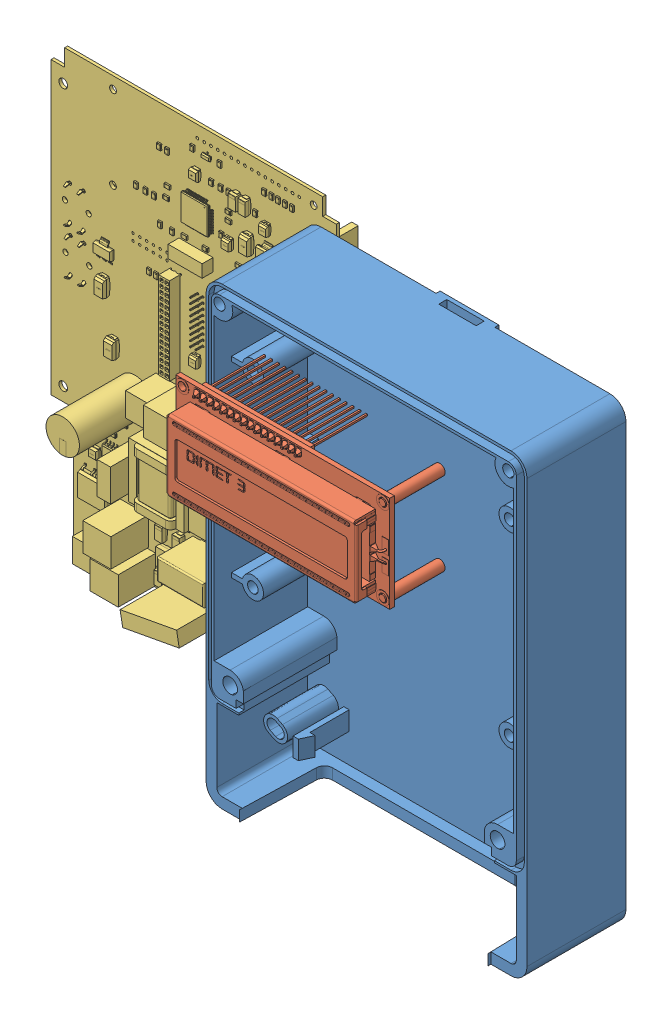
SolidWorks assembly Ensamblaje1, configuration Predeterminado. Lengths in mm.
Overall size (224.33 170.72 94.15).
3 component instances, 3 part files, 3 mates.
Components (placement in the parent):
- DDSF027-base-1: DDSF027-base [Predeterminado] at (0 85 -7) x (-1 0 0) z (0 1 0) size (120 39.5 170)
- General_Display_Ensamble_Parte-1: General_Display_Ensamble_Parte [Predeterminado] at (-7.5039 137.789 52.1227) x (1 0 0) z (0 -1 0) size (80 33.4 36)
- BETESTUNI_01-2: BETESTUNI_01 [Predeterminado] at (-164.851 12.6034 -16.3577) size (110.11 157.73 42.99)
Mates (geometry in assembly coordinates):
- Paralelo1: parallel: plane of assembly through (0 0 0) normal (1 0 0); plane of DDSF027-base-1 through (60 6 31) normal (1 0 0); plane of assembly
- Coincidente1: coincident: point of assembly; moEndPointRef_w of DDSF027-base-1; point of assembly
- Paralelo2: parallel: plane of assembly through (0 0 0) normal (0 0 1); plane of DDSF027-base-1 through (-54 164 -7) normal (0 0 -1); plane of assembly
